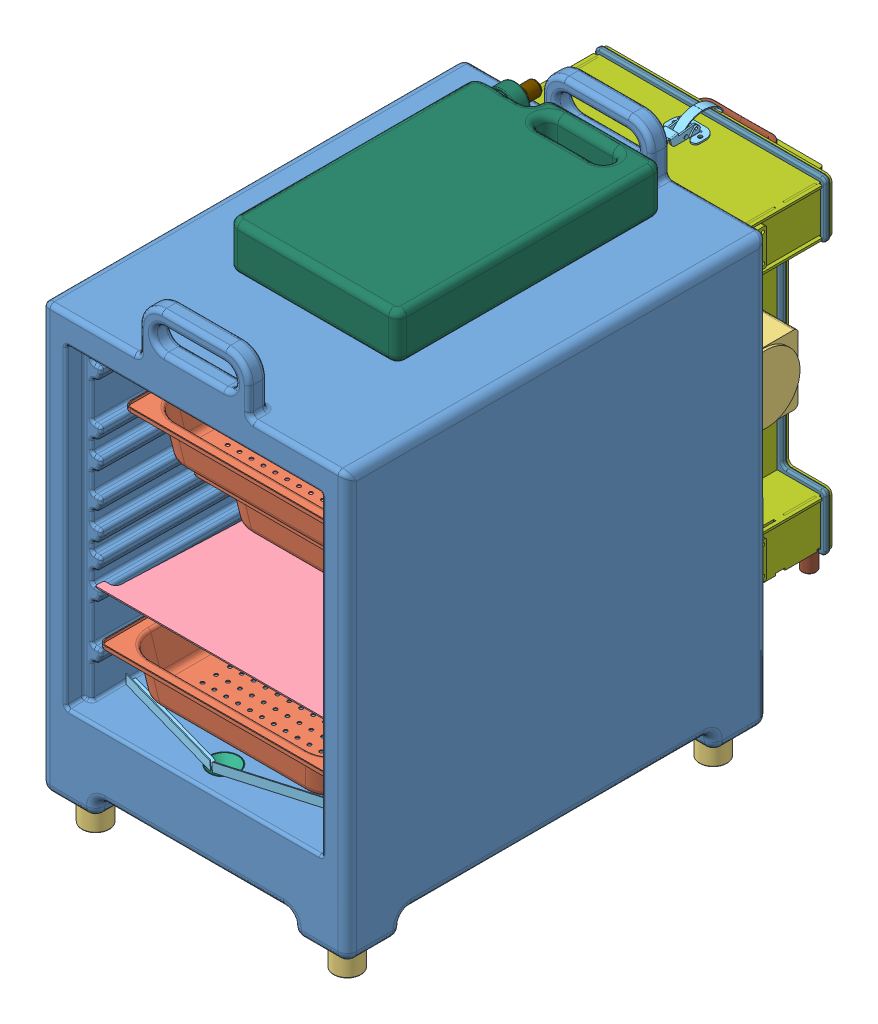
SolidWorks assembly FMT.201, configuration FULL ASSEMBLY. Lengths in mm. (continued)
Mates (geometry in assembly coordinates): (continued)
- Coincident111: coincident: plane of FMT.101-1 through (151.13 109.22 -726.6686) normal (0 -1 0); plane of FMT.202-1 through (0 109.22 -584.2) normal (0 1 0)
- Coincident112: coincident: plane of 9602K410_CORROSION-RESISTANT EQUIPMENT-COOLING FAN-1 through (-52.5145 289.8918 -607.7113) normal (0 1 0); plane of Heating Element-1 through (-2.4765 289.8918 -660.3873) normal (0 -1 0)
- Concentric42: concentric: cylinder of 9602K410_CORROSION-RESISTANT EQUIPMENT-COOLING FAN-1 through (-52.5145 251.8918 -712.7113) axis (0 1 0) radius 2.25; cylinder of Heating Element-1 through (-52.5145 289.8918 -712.7113) axis (0 1 0) radius 2.413
- Parallel19: parallel: plane of 9602K410_CORROSION-RESISTANT EQUIPMENT-COOLING FAN-1 through (-60.0145 82.1862 -607.7113) normal (-1 0 0); plane of Heating Element-1 through (-63.8175 314.0218 -720.0773) normal (-1 0 0)
- Coincident113: coincident: plane of FMT.101-1 through (-151.13 553.72 -726.6686) normal (0 0 -1); plane of 91830A101_18-8 STAINLESS STEEL KNURLED HEAD THUMB SCREW-1 through (142.875 523.24 -726.6686) normal (0 0 1)
- Concentric43: concentric: cylinder of FMT.101-1 through (142.875 523.24 -726.6686) axis (0 0 1) radius 1.4732; cylinder of 91830A101_18-8 STAINLESS STEEL KNURLED HEAD THUMB SCREW-1 through (142.875 523.24 -729.8436) axis (0 0 1) radius 3.175
- Coincident114: coincident: plane of 91830A101_18-8 STAINLESS STEEL KNURLED HEAD THUMB SCREW-1 through (142.875 523.24 -732.2249) normal (0 0 -1); plane of 91830A101_18-8 STAINLESS STEEL KNURLED HEAD THUMB SCREW-2 through (-142.875 523.24 -732.2249) normal (0 0 -1)
- Concentric44: concentric: cylinder of FMT.101-1 through (-142.875 523.24 -726.6686) axis (0 0 1) radius 1.4732; cylinder of 91830A101_18-8 STAINLESS STEEL KNURLED HEAD THUMB SCREW-2 through (-142.875 523.24 -729.8436) axis (0 0 1) radius 3.175
- Coincident115: coincident: plane of 91830A101_18-8 STAINLESS STEEL KNURLED HEAD THUMB SCREW-5 through (85.725 436.88 -732.2249) normal (0 0 -1); plane of 91830A101_18-8 STAINLESS STEEL KNURLED HEAD THUMB SCREW-6 through (-85.725 436.88 -732.2249) normal (0 0 -1)
- Coincident116: coincident: plane of 91830A101_18-8 STAINLESS STEEL KNURLED HEAD THUMB SCREW-1 through (142.875 523.24 -732.2249) normal (0 0 -1); plane of 91830A101_18-8 STAINLESS STEEL KNURLED HEAD THUMB SCREW-6 through (-85.725 436.88 -732.2249) normal (0 0 -1)
- Concentric45: concentric: cylinder of 91830A101_18-8 STAINLESS STEEL KNURLED HEAD THUMB SCREW-5 through (85.725 436.88 -729.8436) axis (0 0 1) radius 3.175; circle of 91780A560_ALUM FEM THRDED HEX STANDOFF-5
- Concentric46: concentric: circle of 91780A560_ALUM FEM THRDED HEX STANDOFF-6; cylinder of 91830A101_18-8 STAINLESS STEEL KNURLED HEAD THUMB SCREW-6 through (-85.725 436.88 -729.8436) axis (0 0 1) radius 3.175
- Coincident117: coincident: plane of 91780A560_ALUM FEM THRDED HEX STANDOFF-1 through (142.875 526.9062 -723.6968) normal (0 0 -1); plane of 91780A560_ALUM FEM THRDED HEX STANDOFF-6 through (-85.725 440.5462 -723.6968) normal (0 0 -1)
- Coincident118: coincident: plane of 91780A560_ALUM FEM THRDED HEX STANDOFF-5 through (85.725 440.5462 -723.6968) normal (0 0 -1); plane of 91780A560_ALUM FEM THRDED HEX STANDOFF-6 through (-85.725 440.5462 -723.6968) normal (0 0 -1)
- Concentric47: concentric: circle of FMT.101-1; cylinder of 91830A101_18-8 STAINLESS STEEL KNURLED HEAD THUMB SCREW-5 through (85.725 436.88 -729.8436) axis (0 0 1) radius 3.175
- Concentric48: concentric: cylinder of FMT.101-1 through (-85.725 436.88 -726.6686) axis (0 0 1) radius 1.4732; cylinder of 91830A101_18-8 STAINLESS STEEL KNURLED HEAD THUMB SCREW-6 through (-85.725 436.88 -729.8436) axis (0 0 1) radius 3.175
- Coincident119: coincident: plane of 4946A100_EXPANDABLE LOCKING GROMMETS-1 through (-92.1702 283.6418 -660.1968) normal (1 0 0); plane of 4946A100_EXPANDABLE LOCKING GROMMETS-2 through (-92.1702 309.0418 -660.1968) normal (1 0 0)
- Concentric49: concentric: cylinder of FMT.101-1 through (-160.02 283.6418 -660.1968) axis (1 0 0) radius 6.35; cylinder of 4946A100_EXPANDABLE LOCKING GROMMETS-1 through (-95.7262 283.6418 -660.1968) axis (-1 0 0) radius 6.35
- Coincident120: coincident: circle of FMT.101-1; plane of 4946A100_EXPANDABLE LOCKING GROMMETS-1 through (-93.345 290.873 -661.4689) normal (1 0 0)
- Coincident121: coincident: circle of FMT.101-1; cylinder of 4946A100_EXPANDABLE LOCKING GROMMETS-2 through (-95.7262 309.0418 -660.1968) axis (-1 0 0) radius 6.35
- Coincident122: coincident: plane of FMT.101-1 through (0 251.8918 -596.6968) normal (0 1 0); plane of 9602K410_CORROSION-RESISTANT EQUIPMENT-COOLING FAN-1 through (-0.0145 251.8918 -660.2113) normal (0 -1 0)
- Coincident125: coincident: plane of FMT.003-1 through (0 50.8 0) normal (0 -1 0); plane of MCM 4629T35-1 through (-57.15 50.8 -318.135) normal (0 1 0)
- Distance10: distance = 50.8 mm: plane of MCM 4629T35-1 through (-161.925 -6.35 -153.67) normal (-1 0 0); plane of FMT.003-1 through (-212.725 590.55 -584.2) normal (-1 0 0)
- Distance11: distance = 25.4 mm: plane of FMT.003-1 through (-212.725 50.8 -508) normal (0 0 1); plane of MCM 4629T35-1 through (47.625 -6.35 -482.6) normal (0 0 -1)
- Coincident126: coincident: plane of FMT.003-1 through (0 0 -584.2) normal (0 0 -1); plane of 1601N123-1 through (0 523.24 -584.2) normal (0 0 1)
- Width35: width: plane of 1601N123-1 through (-152.4 561.34 -584.2) normal (-1 0 0); plane of 1601N123-1 through (152.4 561.34 -584.2) normal (1 0 0); plane of FMT.101-1 through (-153.67 335.28 -596.6968) normal (-1 0 0); plane of FMT.101-1 through (153.67 335.28 -596.6968) normal (1 0 0)
- Width36: width: plane of 1601N123-1 through (-152.4 485.14 -584.2) normal (0 -1 0); plane of 1601N123-1 through (-152.4 561.34 -584.2) normal (0 1 0); plane of FMT.101-1 through (0 556.26 -596.6968) normal (0 1 0); plane of FMT.101-1 through (0 490.22 -596.6968) normal (0 -1 0)
- Coincident127: coincident: plane of 1601N123-1 through (0 523.24 -593.725) normal (0 0 -1); plane of 1601N123-2 through (0 147.32 -593.725) normal (0 0 -1)
- Coincident128: coincident: plane of 1601N123-1 through (-152.4 561.34 -584.2) normal (-1 0 0); plane of 1601N123-2 through (-152.4 185.42 -584.2) normal (-1 0 0)
- Coincident129: coincident: plane of FMT.202-1 through (0 109.22 -584.2) normal (0 1 0); plane of 1601N123-2 through (-152.4 109.22 -584.2) normal (0 -1 0)
- Coincident130: coincident: plane of FMT.101-1 through (-160.02 335.28 -596.6968) normal (-1 0 0); plane of MCM 1659A7-1 through (-160.02 546.5445 -592.8868) normal (1 0 0)
- Distance12: distance = 26.67 mm: plane of MCM 1659A7-1 through (-166.6875 523.24 -608.1268) normal (0 0 -1); plane of FMT.101-1 through (-160.02 548.64 -634.7968) normal (0 0 -1)
- Width37: width: plane of MCM 1659A7-1 through (-172.72 507.365 -592.8868) normal (0 -1 0); plane of MCM 1659A7-1 through (-172.72 539.115 -592.8868) normal (0 1 0); plane of FMT.101-1 through (-160.02 548.64 -634.7968) normal (0 1 0); plane of FMT.101-1 through (-160.02 497.84 -634.7968) normal (0 -1 0)
- Distance13: distance = 2.54 mm: plane of MCM 1659A7-2 through (-169.545 523.24 -622.3) normal (-1 0 0); plane of MCM 1659A7-1 through (-172.085 507.365 -592.8868) normal (1 0 0)
- Width38: width: plane of MCM 1659A7-2 through (-169.545 540.9819 -591.4136) normal (0 1 0); plane of MCM 1659A7-2 through (-169.545 505.4981 -591.4136) normal (0 -1 0); plane of MCM 1659A7-1 through (-172.72 507.365 -592.8868) normal (0 -1 0); plane of MCM 1659A7-1 through (-172.72 539.115 -592.8868) normal (0 1 0)
- Coincident133: coincident: plane of MCM 1659A7-2 through (-169.545 505.4981 -590.55) normal (0 0 1); plane of FMT.203-2 through (-153.3525 711.581 -590.55) normal (0 0 -1)
- Concentric51: concentric: cylinder of MCM 1659A7-2 through (-166.0525 536.956 -622.3) axis (0 0 1) radius 1.5875; cylinder of FMT.203-2 through (-166.0525 536.956 -584.2) axis (0 0 -1) radius 1.651
- Parallel20: parallel: plane of FMT.003-1 through (-212.725 590.55 -584.2) normal (-1 0 0); plane of FMT.203-2 through (-191.4525 498.221 -584.2) normal (-1 0 0)
- Coincident134: coincident: plane of FMT.003-1 through (0 0 -584.2) normal (0 0 -1); plane of FMT.203-2 through (-153.3525 711.581 -584.2) normal (0 0 1)
- Width39: width: plane of FMT.101-1 through (-160.02 372.5418 -609.3968) normal (0 0 -1); plane of FMT.101-1 through (-160.02 372.5418 -683.0568) normal (0 0 1); plane of GeekTeches Thermoelectric Peltier Refrigeration Cooling System, Radiator Semiconductor Cooler Conduction Module Fan-1 through (93.345 387.7818 -597.9668) normal (0 0 1); plane of GeekTeches Thermoelectric Peltier Refrigeration Cooling System, Radiator Semiconductor Cooler Conduction Module Fan-1 through (93.345 387.7818 -694.4868) normal (0 0 -1)
- Width40: width: plane of GeekTeches Thermoelectric Peltier Refrigeration Cooling System, Radiator Semiconductor Cooler Conduction Module Fan-1 through (93.345 387.7818 -694.4868) normal (0 1 0); plane of GeekTeches Thermoelectric Peltier Refrigeration Cooling System, Radiator Semiconductor Cooler Conduction Module Fan-1 through (93.345 291.2618 -694.4868) normal (0 -1 0); plane of FMT.101-1 through (-160.02 306.5018 -609.3968) normal (0 1 0); plane of FMT.101-1 through (-160.02 372.5418 -609.3968) normal (0 -1 0)
- Coincident135: coincident: plane of FMT.101-1 through (93.345 335.28 -596.6968) normal (1 0 0); plane of GeekTeches Thermoelectric Peltier Refrigeration Cooling System, Radiator Semiconductor Cooler Conduction Module Fan-1 through (93.345 339.5218 -646.2268) normal (-1 0 0)
- Width41: width: plane of FMT.011-1 through (-77.47 479.8818 -726.0409) normal (-1 0 0); plane of FMT.011-1 through (77.47 479.8818 -726.0409) normal (1 0 0); plane of FMT.101-1 through (93.345 335.28 -596.6968) normal (1 0 0); plane of FMT.101-1 through (-93.345 335.28 -596.6968) normal (-1 0 0)
- Coincident136: coincident: plane of FMT.203-2 through (-191.4525 549.021 -584.2) normal (0 1 0); plane of FMT.203-4 through (191.5556 549.021 -584.2) normal (0 1 0)
- Coincident137: coincident: plane of FMT.203-2 through (-153.3525 711.581 -590.55) normal (0 0 -1); plane of FMT.203-4 through (153.4556 335.661 -590.55) normal (0 0 -1)
- Concentric52: concentric: circle of 91115A834_18-8 SS FEM THRDED HEX STANDOFF-1; circle of 92949A148_18-8 SS BUTTON-HEAD SOCKET CAP SCREW-5
- Coincident141: coincident: plane of 91115A834_18-8 SS FEM THRDED HEX STANDOFF-1 through (65.3331 375.945 -723.6968) normal (0 0 -1); plane of 91115A834_18-8 SS FEM THRDED HEX STANDOFF-3 through (3.6662 372.77 -723.6968) normal (0 0 -1)
- Coincident142: coincident: plane of 91115A834_18-8 SS FEM THRDED HEX STANDOFF-2 through (-61.6669 375.945 -723.6968) normal (0 0 -1); plane of 91115A834_18-8 SS FEM THRDED HEX STANDOFF-3 through (3.6662 372.77 -723.6968) normal (0 0 -1)
- Coincident143: coincident: plane of 92949A148_18-8 SS BUTTON-HEAD SOCKET CAP SCREW-5 through (61.8945 372.0672 -728.5228) normal (0 0 -1); plane of 92949A148_18-8 SS BUTTON-HEAD SOCKET CAP SCREW-6 through (-1.6055 372.0672 -728.5228) normal (0 0 -1)
- Coincident144: coincident: plane of 92949A148_18-8 SS BUTTON-HEAD SOCKET CAP SCREW-6 through (-1.6055 372.0672 -728.5228) normal (0 0 -1); plane of 92949A148_18-8 SS BUTTON-HEAD SOCKET CAP SCREW-7 through (-65.1871 373.2447 -728.5228) normal (0 0 -1)
- Concentric53: concentric: circle of 91115A834_18-8 SS FEM THRDED HEX STANDOFF-2; cylinder of 92949A148_18-8 SS BUTTON-HEAD SOCKET CAP SCREW-7 through (-63.5 372.77 -728.5228) axis (0 0 -1) radius 3.3274
- Concentric54: concentric: circle of 91115A834_18-8 SS FEM THRDED HEX STANDOFF-3; cylinder of 92949A148_18-8 SS BUTTON-HEAD SOCKET CAP SCREW-6 through (0 372.77 -728.5228) axis (0 0 -1) radius 3.3274
- Concentric55: concentric: cylinder of FMT.101-1 through (63.5 372.77 -593.725) axis (0 0 -1) radius 1.5; cylinder of 92949A148_18-8 SS BUTTON-HEAD SOCKET CAP SCREW-5 through (63.5 372.77 -728.5228) axis (0 0 -1) radius 3.3274
- Coincident146: coincident: plane of FMT.101-1 through (-151.13 553.72 -723.6968) normal (0 0 1); plane of 91115A834_18-8 SS FEM THRDED HEX STANDOFF-1 through (65.3331 375.945 -723.6968) normal (0 0 -1)
- Concentric56: concentric: cylinder of FMT.101-1 through (0 372.77 -593.725) axis (0 0 -1) radius 1.5; cylinder of 92949A148_18-8 SS BUTTON-HEAD SOCKET CAP SCREW-6 through (0 372.77 -728.5228) axis (0 0 -1) radius 3.3274
- Concentric57: concentric: cylinder of FMT.101-1 through (-63.5 372.77 -593.725) axis (0 0 -1) radius 1.5; cylinder of 92949A148_18-8 SS BUTTON-HEAD SOCKET CAP SCREW-7 through (-63.5 372.77 -728.5228) axis (0 0 -1) radius 3.3274
- Parallel22: parallel: plane of FMT.101-1 through (81 375.92 -593.725) normal (0 1 0); plane of 91115A834_18-8 SS FEM THRDED HEX STANDOFF-1 through (65.3331 375.945 -647.4968) normal (0 1 0)
- Coincident147: coincident: plane of 91115A834_18-8 SS FEM THRDED HEX STANDOFF-1 through (65.3331 375.945 -647.4968) normal (0 1 0); plane of 91115A834_18-8 SS FEM THRDED HEX STANDOFF-3 through (1.8331 375.945 -647.4968) normal (0 1 0)
- Coincident148: coincident: plane of 91115A834_18-8 SS FEM THRDED HEX STANDOFF-2 through (-61.6669 375.945 -647.4968) normal (0 1 0); plane of 91115A834_18-8 SS FEM THRDED HEX STANDOFF-3 through (1.8331 375.945 -647.4968) normal (0 1 0)
- Coincident149: coincident: plane of FMT.011-1 through (0 375.945 -686.4169) normal (0 -1 0); plane of 91115A834_18-8 SS FEM THRDED HEX STANDOFF-1 through (65.3331 375.945 -647.4968) normal (0 1 0)
- Coincident150: coincident: plane of FMT.101-1 through (-151.13 553.72 -726.6686) normal (0 0 -1); plane of 92949A148_18-8 SS BUTTON-HEAD SOCKET CAP SCREW-7 through (-66.703 373.6712 -726.6686) normal (0 0 1)
- Coincident151: coincident: plane of FITNATE Mist Maker-1 through (0.0034 378.9168 -686.4169) normal (0 -1 0); plane of FITNATE Mist Maker-2 through (57.1534 378.9168 -686.4169) normal (0 -1 0)
- Coincident152: coincident: circle of FMT.204-1; cone of FITNATE Mist Maker-1 through (-28.575 409.6508 -686.4169) axis (0 1 0)
- Coincident153: coincident: circle of FMT.204-1; cone of FITNATE Mist Maker-2 through (28.575 409.6508 -686.4169) axis (0 1 0)
- Width42: width: plane of FMT.011-1 through (-77.47 378.9168 -648.0629) normal (0 0 -1); plane of FMT.011-1 through (-77.47 378.9168 -724.7709) normal (0 0 1); plane of FMT.204-1 through (0.7958 417.1121 -724.7669) normal (0 0 -1); plane of FMT.204-1 through (0.7958 417.1121 -648.0669) normal (0 0 1)
- Width43: width: plane of FMT.204-1 through (-76.35 417.1121 -867.9228) normal (-1 0 0); plane of FMT.204-1 through (76.35 417.1121 -867.9228) normal (1 0 0); plane of FMT.011-1 through (77.47 302.1983 -648.0629) normal (1 0 0); plane of FMT.011-1 through (-77.47 302.1983 -648.0629) normal (-1 0 0)
- Coincident154: coincident: plane of FMT.011-1 through (0 378.9168 -686.4169) normal (0 1 0); plane of FITNATE Mist Maker-1 through (0.0034 378.9168 -686.4169) normal (0 -1 0)
- Coincident157: coincident: plane of FMT.204-1 through (0.7958 420.0838 -867.9228) normal (0 1 0); plane of 91115A135_18-8 SS FEM THRDED HEX STANDOFF-1 through (50 420.0838 -690.0831) normal (0 -1 0)
- Concentric62: concentric: cylinder of FMT.204-1 through (50 100.5519 -686.4169) axis (0 1 0) radius 1.8288; circle of 91115A135_18-8 SS FEM THRDED HEX STANDOFF-1
- Coincident159: coincident: plane of 91115A135_18-8 SS FEM THRDED HEX STANDOFF-1 through (50 458.1839 -690.0831) normal (0 1 0); plane of 91115A135_18-8 SS FEM THRDED HEX STANDOFF-2 through (-50 458.1839 -690.0831) normal (0 1 0)
- Concentric63: concentric: cylinder of FMT.204-1 through (-50 100.5519 -686.4169) axis (0 1 0) radius 1.8288; circle of 91115A135_18-8 SS FEM THRDED HEX STANDOFF-2
- Coincident160: coincident: plane of 92949A537_18-8 SS BUTTON-HEAD SOCKET CAP SCREW-5 through (-48.5987 437.2864 -724.7709) normal (0 0 -1); plane of 92949A537_18-8 SS BUTTON-HEAD SOCKET CAP SCREW-6 through (56.1763 437.2864 -724.7709) normal (0 0 -1)
- Coincident161: coincident: plane of FMT.011-1 through (-77.47 378.9168 -724.7709) normal (0 0 1); plane of 92949A537_18-8 SS BUTTON-HEAD SOCKET CAP SCREW-6 through (56.1763 437.2864 -724.7709) normal (0 0 -1)
- Concentric64: concentric: circle of 1661A100_LOAD-RATED PULL HANDLE WITH THREADED HOLES-3; circle of 92949A537_18-8 SS BUTTON-HEAD SOCKET CAP SCREW-5
- Concentric65: concentric: circle of 1661A100_LOAD-RATED PULL HANDLE WITH THREADED HOLES-3; cylinder of 92949A537_18-8 SS BUTTON-HEAD SOCKET CAP SCREW-6 through (52.3875 441.3418 -721.4181) axis (0 0 1) radius 5.5499
- Concentric66: concentric: cylinder of FMT.011-1 through (52.3875 441.3418 -723.0691) axis (0 0 -1) radius 3.175; cylinder of 92949A537_18-8 SS BUTTON-HEAD SOCKET CAP SCREW-6 through (52.3875 441.3418 -721.4181) axis (0 0 1) radius 5.5499
- Concentric67: concentric: cylinder of FMT.011-1 through (-52.3875 441.3418 -723.0691) axis (0 0 -1) radius 3.175; cylinder of 92949A537_18-8 SS BUTTON-HEAD SOCKET CAP SCREW-5 through (-52.3875 441.3418 -721.4181) axis (0 0 1) radius 5.5499
- Coincident162: coincident: plane of FMT.011-1 through (-77.47 378.9168 -726.0409) normal (0 0 -1); plane of 1661A100_LOAD-RATED PULL HANDLE WITH THREADED HOLES-3 through (-46.0375 431.0231 -726.0409) normal (0 0 1)
- Coincident164: coincident: plane of FMT.101-1 through (93.345 335.28 -596.6968) normal (1 0 0); plane of 4946A100_EXPANDABLE LOCKING GROMMETS-3 through (93.345 283.6418 -652.8546) normal (-1 0 0)
- Concentric70: concentric: cylinder of FMT.101-1 through (-160.02 283.6418 -660.1968) axis (1 0 0) radius 6.35; cylinder of 4946A100_EXPANDABLE LOCKING GROMMETS-3 through (95.7262 283.6418 -660.1968) axis (1 0 0) radius 7.3422
- Coincident165: coincident: plane of FMT.101-1 through (0 556.26 -596.6968) normal (0 1 0); plane of 1863A210_DRAW LATCH-2 through (-12.0223 556.26 -691.8409) normal (0 -1 0)
- Concentric71: concentric: cylinder of FMT.101-1 through (17.4625 109.22 -685.0126) axis (0 1 0) radius 1.905; cylinder of 1863A210_DRAW LATCH-2 through (17.4625 558.292 -685.0126) axis (0 -1 0) radius 2.7686
- Concentric72: concentric: cylinder of FMT.101-1 through (-17.4625 109.22 -685.0126) axis (0 1 0) radius 1.905; cylinder of 1863A210_DRAW LATCH-2 through (-17.4625 558.292 -685.0126) axis (0 -1 0) radius 2.7686
- Coincident166: coincident: plane of FMT.101-1 through (0 114.3 -596.6968) normal (0 -1 0); plane of 1863A210_DRAW LATCH-1 through (12.0223 114.3 -691.8409) normal (0 1 0)
- Concentric73: concentric: cylinder of FMT.101-1 through (17.4625 109.22 -685.0126) axis (0 1 0) radius 1.905; cylinder of 1863A210_DRAW LATCH-1 through (17.4625 112.268 -685.0126) axis (0 1 0) radius 2.7686
- Concentric74: concentric: cylinder of FMT.101-1 through (-17.4625 109.22 -685.0126) axis (0 1 0) radius 1.905; cylinder of 1863A210_DRAW LATCH-1 through (-17.4625 112.268 -685.0126) axis (0 1 0) radius 2.7686
- Coincident167: coincident: plane of FMT.101-1 through (0 114.3 -596.6968) normal (0 -1 0); plane of 9540K731 Rubber Bumper with Unthreaded Hole-1 through (142.875 114.3 -710.9968) normal (0 1 0)
- Coincident168: coincident: plane of 9540K731 Rubber Bumper with Unthreaded Hole-2 through (-142.875 114.3 -710.9968) normal (0 1 0); plane of 9540K731 Rubber Bumper with Unthreaded Hole-3 through (142.875 114.3 -619.125) normal (0 1 0)
- Coincident169: coincident: plane of 9540K731 Rubber Bumper with Unthreaded Hole-3 through (142.875 114.3 -619.125) normal (0 1 0); circle of 9540K731 Rubber Bumper with Unthreaded Hole-4
- Coincident170: coincident: plane of 9540K731 Rubber Bumper with Unthreaded Hole-1 through (142.875 114.3 -710.9968) normal (0 1 0); plane of 9540K731 Rubber Bumper with Unthreaded Hole-2 through (-142.875 114.3 -710.9968) normal (0 1 0)
- Concentric75: concentric: cylinder of FMT.101-1 through (-142.875 561.34 -619.125) axis (0 -1 0) radius 1.9844; cylinder of 9540K731 Rubber Bumper with Unthreaded Hole-4 through (-142.875 88.9 -619.125) axis (0 1 0) radius 9.525
- Concentric76: concentric: cylinder of FMT.101-1 through (142.875 561.34 -619.125) axis (0 -1 0) radius 1.9844; cylinder of 9540K731 Rubber Bumper with Unthreaded Hole-3 through (142.875 88.9 -619.125) axis (0 1 0) radius 9.525
- Concentric77: concentric: cylinder of FMT.101-1 through (142.875 561.34 -710.9968) axis (0 -1 0) radius 1.9844; cylinder of 9540K731 Rubber Bumper with Unthreaded Hole-1 through (142.875 88.9 -710.9968) axis (0 1 0) radius 9.525
- Concentric78: concentric: cylinder of FMT.101-1 through (-142.875 561.34 -710.9968) axis (0 -1 0) radius 1.9844; cylinder of 9540K731 Rubber Bumper with Unthreaded Hole-2 through (-142.875 88.9 -710.9968) axis (0 1 0) radius 9.525
- Concentric79: concentric: cylinder of 9540K731 Rubber Bumper with Unthreaded Hole-2 through (-142.875 95.25 -710.9968) axis (0 -1 0) radius 4.7625; cylinder of 92949A153_18-8 SS BUTTON-HEAD SOCKET CAP SCREW-1 through (-142.875 93.3958 -710.9968) axis (0 -1 0) radius 3.3274
- Coincident171: coincident: plane of 92949A153_18-8 SS BUTTON-HEAD SOCKET CAP SCREW-1 through (-143.8339 93.3958 -709.5298) normal (0 -1 0); plane of 92949A153_18-8 SS BUTTON-HEAD SOCKET CAP SCREW-2 through (-143.8336 93.3958 -617.6578) normal (0 -1 0)
- Coincident172: coincident: plane of 92949A153_18-8 SS BUTTON-HEAD SOCKET CAP SCREW-2 through (-143.8336 93.3958 -617.6578) normal (0 -1 0); circle of 92949A153_18-8 SS BUTTON-HEAD SOCKET CAP SCREW-4
- Coincident174: coincident: plane of 92949A153_18-8 SS BUTTON-HEAD SOCKET CAP SCREW-3 through (141.9164 93.3958 -617.6578) normal (0 -1 0); plane of 92949A153_18-8 SS BUTTON-HEAD SOCKET CAP SCREW-4 through (141.9164 93.3958 -709.5296) normal (0 -1 0)
- Coincident175: coincident: plane of 9540K731 Rubber Bumper with Unthreaded Hole-2 through (-142.875 95.25 -710.9968) normal (0 -1 0); plane of 92949A153_18-8 SS BUTTON-HEAD SOCKET CAP SCREW-1 through (-144.6955 95.25 -708.2116) normal (0 1 0)
- Concentric81: concentric: cylinder of 9540K731 Rubber Bumper with Unthreaded Hole-4 through (-142.875 88.9 -619.125) axis (0 1 0) radius 9.525; cylinder of 92949A153_18-8 SS BUTTON-HEAD SOCKET CAP SCREW-2 through (-142.875 93.3958 -619.125) axis (0 -1 0) radius 3.3274
- Concentric82: concentric: cylinder of 9540K731 Rubber Bumper with Unthreaded Hole-1 through (142.875 88.9 -710.9968) axis (0 1 0) radius 9.525; cylinder of 92949A153_18-8 SS BUTTON-HEAD SOCKET CAP SCREW-4 through (142.875 93.3958 -710.9968) axis (0 -1 0) radius 3.3274
- Concentric83: concentric: cylinder of 9540K731 Rubber Bumper with Unthreaded Hole-3 through (142.875 88.9 -619.125) axis (0 1 0) radius 9.525; cylinder of 92949A153_18-8 SS BUTTON-HEAD SOCKET CAP SCREW-3 through (142.875 93.3958 -619.125) axis (0 -1 0) radius 3.3274
- Coincident176: coincident: plane of 91841A007_TYPE 18-8 STAINLESS STEEL HEX NUT-1 through (-146.8438 120.0499 -713.2882) normal (0 1 0); plane of 91841A007_TYPE 18-8 STAINLESS STEEL HEX NUT-4 through (-146.8438 120.0499 -621.4164) normal (0 1 0)
- Coincident177: coincident: plane of 91841A007_TYPE 18-8 STAINLESS STEEL HEX NUT-3 through (138.9062 120.0499 -713.2882) normal (0 1 0); plane of 91841A007_TYPE 18-8 STAINLESS STEEL HEX NUT-4 through (-146.8438 120.0499 -621.4164) normal (0 1 0)
- Coincident178: coincident: plane of 91841A007_TYPE 18-8 STAINLESS STEEL HEX NUT-2 through (138.9062 120.0499 -621.4164) normal (0 1 0); plane of 91841A007_TYPE 18-8 STAINLESS STEEL HEX NUT-3 through (138.9062 120.0499 -713.2882) normal (0 1 0)
- Coincident179: coincident: plane of FMT.101-1 through (0 117.2718 -596.6968) normal (0 1 0); plane of 91841A007_TYPE 18-8 STAINLESS STEEL HEX NUT-1 through (-146.8438 117.2718 -713.2882) normal (0 -1 0)
- Concentric84: concentric: cylinder of 9540K731 Rubber Bumper with Unthreaded Hole-2 through (-142.875 88.9 -710.9968) axis (0 1 0) radius 9.525; circle of 91841A007_TYPE 18-8 STAINLESS STEEL HEX NUT-1
- Concentric85: concentric: cylinder of 9540K731 Rubber Bumper with Unthreaded Hole-4 through (-142.875 88.9 -619.125) axis (0 1 0) radius 9.525; circle of 91841A007_TYPE 18-8 STAINLESS STEEL HEX NUT-4
- Concentric86: concentric: cylinder of 9540K731 Rubber Bumper with Unthreaded Hole-1 through (142.875 88.9 -710.9968) axis (0 1 0) radius 9.525; circle of 91841A007_TYPE 18-8 STAINLESS STEEL HEX NUT-3
- Concentric87: concentric: cylinder of 9540K731 Rubber Bumper with Unthreaded Hole-3 through (142.875 88.9 -619.125) axis (0 1 0) radius 9.525; circle of 91841A007_TYPE 18-8 STAINLESS STEEL HEX NUT-2
- Coincident180: coincident: plane of FMT.101-1 through (0 556.26 -596.6968) normal (0 1 0); plane of 93085K11 Surface-Mount, Hollow, 375 Wide, 1875 ID Rubber Seal-1 through (-153.67 556.26 -723.6968) normal (0 -1 0)
- Coincident181: coincident: plane of FMT.101-1 through (153.67 335.28 -596.6968) normal (1 0 0); plane of 93085K11 Surface-Mount, Hollow, 375 Wide, 1875 ID Rubber Seal-1 through (153.67 556.26 -723.6968) normal (-1 0 0)
- Coincident182: coincident: plane of FMT.101-1 through (-151.13 553.72 -723.6968) normal (0 0 1); plane of 93085K11 Surface-Mount, Hollow, 375 Wide, 1875 ID Rubber Seal-1 through (0 335.28 -723.6968) normal (0 0 -1)
- Coincident183: coincident: plane of FMT.003-1 through (-212.725 590.55 -584.2) normal (0 1 0); plane of 1542N2 HDPE TANK-1 through (0 590.55 -349.25) normal (0 -1 0)
- Coincident185: coincident: plane of FMT.011-1 through (-77.47 378.9168 -724.7709) normal (0 0 1); plane of 5779K162_PUSH-TO-CONNECT TUBE FITTING FOR AIR-1 through (-69.47 482.6623 -724.7709) normal (0 0 -1)
- Concentric89: concentric: cylinder of FMT.011-1 through (-59.47 465.3418 -646.7919) axis (0 0 -1) radius 7.112; cylinder of 5779K162_PUSH-TO-CONNECT TUBE FITTING FOR AIR-1 through (-59.47 465.3418 -704.8319) axis (0 0 -1) radius 8.8392
- Parallel23: parallel: plane of FMT.011-1 through (-77.47 302.1983 -648.0629) normal (-1 0 0); plane of 5779K162_PUSH-TO-CONNECT TUBE FITTING FOR AIR-1 through (-69.47 471.1153 -719.7709) normal (-1 0 0)
- Concentric90: concentric: cylinder of 5779K162_PUSH-TO-CONNECT TUBE FITTING FOR AIR-1 through (-59.47 465.3418 -706.3976) axis (0 0 -1) radius 4.7282; cylinder of 5779K455_PUSH-TO-CONNECT TUBE FITTING FOR AIR-1 through (-59.47 465.3418 -759.9499) axis (0 0 1) radius 8.8392
- Angle1: planar angle = 0.523599 rad: plane of 5779K162_PUSH-TO-CONNECT TUBE FITTING FOR AIR-1 through (-69.47 471.1153 -719.7709) normal (-1 0 0); plane of 5779K455_PUSH-TO-CONNECT TUBE FITTING FOR AIR-1 through (-70.4397 465.3418 -742.0429) normal (-0.866025 -0.5 0)
- Coincident186: coincident: plane of FMT.011-1 through (-77.47 378.9168 -726.0409) normal (0 0 -1); plane of 5779K455_PUSH-TO-CONNECT TUBE FITTING FOR AIR-1 through (-59.47 465.3418 -726.0409) normal (0 0 1)
- Concentric91: concentric: cylinder of 1542N2 HDPE TANK-1 through (-92.075 622.3 -538.48) axis (0 0 1) radius 7.112; cylinder of 5779K119_PUSH-TO-CONNECT TUBE FITTING FOR AIR-1 through (-92.075 622.3 -528.2743) axis (0 0 1) radius 9.9
- Coincident187: coincident: plane of 1542N2 HDPE TANK-1 through (-92.075 622.3 -538.48) normal (0 0 -1); plane of 5779K119_PUSH-TO-CONNECT TUBE FITTING FOR AIR-1 through (-73.952 609.8278 -538.48) normal (0 0 1)
- Concentric92: concentric: cylinder of 5779K119_PUSH-TO-CONNECT TUBE FITTING FOR AIR-1 through (-92.075 622.3 -528.2743) axis (0 0 1) radius 9.9; circle of 50785K142_MED-PRESSURE BRASS THREADED PIPE FITTING-1
- Coincident188: coincident: plane of 1542N2 HDPE TANK-1 through (-92.075 622.3 -535.94) normal (0 0 1); plane of 50785K142_MED-PRESSURE BRASS THREADED PIPE FITTING-1 through (-80.157 617.5449 -535.94) normal (0 0 -1)
- Width44: width: plane of 1542N2 HDPE TANK-1 through (117.475 654.05 -533.4) normal (1 0 0); plane of 1542N2 HDPE TANK-1 through (-117.475 654.05 -533.4) normal (-1 0 0); plane of FMT.003-1 through (-212.725 590.55 -584.2) normal (-1 0 0); plane of FMT.003-1 through (212.725 590.55 -584.2) normal (1 0 0)
- Distance14: distance = 50.8 mm: plane of FMT.003-1 through (0 0 -584.2) normal (0 0 -1); plane of 1542N2 HDPE TANK-1 through (-117.475 654.05 -533.4) normal (0 0 -1)
- Concentric93: concentric: cylinder of FMT.205-1 through (-50 464.5339 -686.4169) axis (0 -1 0) radius 1.8288; circle of 91115A135_18-8 SS FEM THRDED HEX STANDOFF-2
- Concentric94: concentric: cylinder of FMT.205-1 through (50 464.5339 -686.4169) axis (0 -1 0) radius 1.8288; circle of 91115A135_18-8 SS FEM THRDED HEX STANDOFF-1
- Coincident190: coincident: plane of FMT.205-1 through (-0.7958 458.1839 -504.9109) normal (0 -1 0); plane of 91115A135_18-8 SS FEM THRDED HEX STANDOFF-1 through (50 458.1839 -690.0831) normal (0 1 0)
- Coincident191: coincident: plane of FMT.205-1 through (-0.7958 464.5339 -504.9109) normal (0 1 0); plane of 92949A148_18-8 SS BUTTON-HEAD SOCKET CAP SCREW-8 through (50 464.5339 -683.0895) normal (0 -1 0)
- Concentric95: concentric: cylinder of FMT.205-1 through (50 464.5339 -686.4169) axis (0 -1 0) radius 1.8288; cylinder of 92949A148_18-8 SS BUTTON-HEAD SOCKET CAP SCREW-8 through (50 466.3881 -686.4169) axis (0 1 0) radius 3.3274
- Coincident192: coincident: plane of 92949A148_18-8 SS BUTTON-HEAD SOCKET CAP SCREW-8 through (50 466.3881 -684.6643) normal (0 1 0); plane of 92949A148_18-8 SS BUTTON-HEAD SOCKET CAP SCREW-9 through (-50 466.3881 -684.6643) normal (0 1 0)
- Concentric96: concentric: cylinder of FMT.205-1 through (-50 464.5339 -686.4169) axis (0 -1 0) radius 1.8288; cylinder of 92949A148_18-8 SS BUTTON-HEAD SOCKET CAP SCREW-9 through (-50 466.3881 -686.4169) axis (0 1 0) radius 3.3274
- Coincident193: coincident: plane of 92949A148_18-8 SS BUTTON-HEAD SOCKET CAP SCREW-10 through (48.1801 417.1121 -683.6313) normal (0 1 0); plane of 92949A148_18-8 SS BUTTON-HEAD SOCKET CAP SCREW-11 through (-51.8199 417.1121 -683.6313) normal (0 1 0)
- Coincident195: coincident: plane of FMT.204-1 through (0.7958 417.1121 -867.9228) normal (0 -1 0); plane of 92949A148_18-8 SS BUTTON-HEAD SOCKET CAP SCREW-10 through (48.1801 417.1121 -683.6313) normal (0 1 0)
- Concentric97: concentric: cylinder of FMT.204-1 through (50 100.5519 -686.4169) axis (0 1 0) radius 1.8288; cylinder of 92949A148_18-8 SS BUTTON-HEAD SOCKET CAP SCREW-10 through (50 415.2578 -686.4169) axis (0 -1 0) radius 3.3274
- Concentric98: concentric: cylinder of FMT.204-1 through (-50 100.5519 -686.4169) axis (0 1 0) radius 1.8288; cylinder of 92949A148_18-8 SS BUTTON-HEAD SOCKET CAP SCREW-11 through (-50 415.2578 -686.4169) axis (0 -1 0) radius 3.3274
